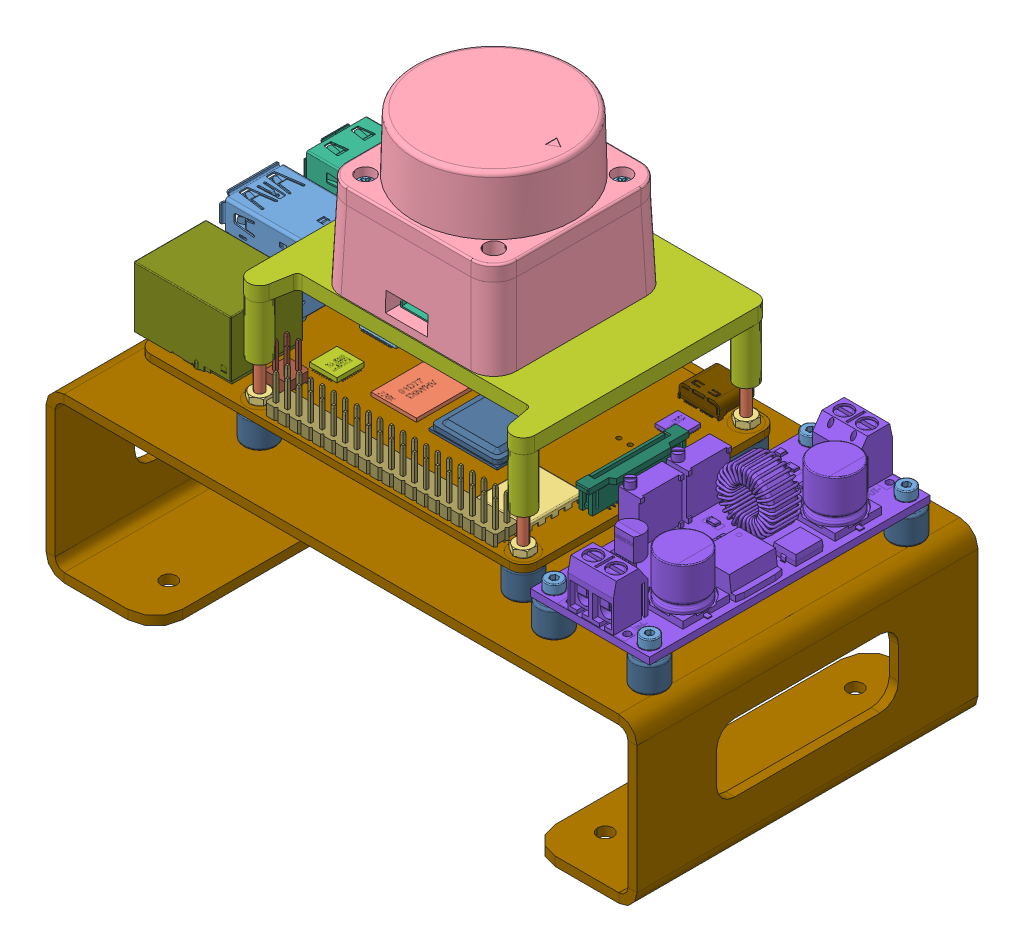
SolidWorks assembly 3rdFloorAssembly, configuration Default. Lengths in mm.
Overall size (130 100.19 75).
53 component instances, 28 part files, 56 mates.
Components (placement in the parent):
- socket head cap screw 4762_din-1: socket head cap screw 4762_din [EN ISO 4762 M2 x 12 - 12S] at (37.5 45.65 -28.25) x (0 -1 0) z (0 0 1) size (14 3.8 3.8)
- socket head cap screw 4762_din-2: socket head cap screw 4762_din [EN ISO 4762 M2 x 12 - 12S] at (58.5 45.65 -28.25) x (0 -1 0) z (0 0 1) size (14 3.8 3.8)
- socket head cap screw 4762_din-3: socket head cap screw 4762_din [EN ISO 4762 M2 x 12 - 12S] at (58.5 45.65 28.25) x (0 -1 0) z (0 0 1) size (14 3.8 3.8)
- socket head cap screw 4762_din-4: socket head cap screw 4762_din [EN ISO 4762 M2 x 12 - 12S] at (37.5 45.65 28.25) x (0 -1 0) z (0 0 1) size (14 3.8 3.8)
- socket head cap screw_iso-1: socket head cap screw_iso [ISO 4762 M2 x 20 - 20C] at (-31 32 -24.5) x (0 1 0) z (0 0 1) size (22 3.8 3.8)
- socket head cap screw_iso-2: socket head cap screw_iso [ISO 4762 M2 x 20 - 20C] at (-31 32 24.5) x (0 1 0) z (0 0 1) size (22 3.8 3.8)
- socket head cap screw_iso-3: socket head cap screw_iso [ISO 4762 M2 x 20 - 20C] at (27 32 -24.5) x (0 1 0) z (0 0 1) size (22 3.8 3.8)
- socket head cap screw_iso-4: socket head cap screw_iso [ISO 4762 M2 x 20 - 20C] at (27 32 24.5) x (0 1 0) z (0 0 1) size (22 3.8 3.8)
- hex nut style 1 gradeab_iso-1: hex nut style 1 gradeab_iso [ISO - 4032 - M2 - W - C] at (-31 45.19 -24.5) x (1 0 0) z (0 1 0) size (4 4.62 1.6)
- hex nut style 1 gradeab_iso-2: hex nut style 1 gradeab_iso [ISO - 4032 - M2 - W - C] at (27 45.19 -24.5) x (1 0 0) z (0 1 0) size (4 4.62 1.6)
- hex nut style 1 gradeab_iso-3: hex nut style 1 gradeab_iso [ISO - 4032 - M2 - W - C] at (-31 45.19 24.5) x (1 0 0) z (0 1 0) size (4 4.62 1.6)
- hex nut style 1 gradeab_iso-4: hex nut style 1 gradeab_iso [ISO - 4032 - M2 - W - C] at (27 45.19 24.5) x (1 0 0) z (0 1 0) size (4 4.62 1.6)
- hex nut style 1 gradeab_iso-5: hex nut style 1 gradeab_iso [ISO - 4032 - M2 - W - C] at (58.5 32.4 -28.25) x (1 0 0) z (0 -1 0) size (4 4.62 1.6)
- hex nut style 1 gradeab_iso-6: hex nut style 1 gradeab_iso [ISO - 4032 - M2 - W - C] at (37.5 32.4 -28.25) x (1 0 0) z (0 -1 0) size (4 4.62 1.6)
- hex nut style 1 gradeab_iso-7: hex nut style 1 gradeab_iso [ISO - 4032 - M2 - W - C] at (37.5 32.4 28.25) x (1 0 0) z (0 -1 0) size (4 4.62 1.6)
- hex nut style 1 gradeab_iso-8: hex nut style 1 gradeab_iso [ISO - 4032 - M2 - W - C] at (58.5 32.4 28.25) x (1 0 0) z (0 -1 0) size (4 4.62 1.6)
- LD06_Assembly-1: LD06_Assembly [Default] at (-60.828 42.1202 31.9351) x (0 0 -1) z (1 0 0) size (54 48.5 63)
  - LD06_LiDAR-1: LD06_LiDAR [Default] at (15.6414 21.3154 28.1688) size (38.59 33.3 38.59)
    - LD06_LiDAR-1: LD06_LiDAR [Default] at (16.3187 3.4544 28.6342) size (38.59 33.3 38.59)
    - JIS_B1111_M2x6.step-1: JIS_B1111_M2x6.step [Default] at (30.4187 21.1806 42.7342) x (1 0 0) z (0 1 0) size (3.5 3.5 7.3)
    - JIS_B1111_M2x6.step-2: JIS_B1111_M2x6.step [Default] at (2.2187 21.1806 14.5342) x (1 0 0) z (0 1 0) size (3.5 3.5 7.3)
    - jst-1.5mm-4P.step-1: jst-1.5mm-4P.step [Default] at (4.0237 7.1794 28.6342) x (0 0 -1) z (0 1 0) size (7.5 7.2 3.5)
  - LD06_PiBracket-1: LD06_PiBracket [Default] at (31.9351 21.5698 58.828) x (0 0 1) z (-1 0 0) size (63 27 54)
- dc-dc-5a-cc-merged-1: dc-dc-5a-cc-merged [Default] at (48 43.6 0) x (0 0 -1) z (1 0 0) size (61.7 17.87 26.2)
- Raspberry Pi 4 Model B-1: Raspberry Pi 4 Model B [Default] at (-12 42.8 0) x (-1 0 0) z (0 0 -1) size (88.99 19.9 58.4)
  - PCB, RPi4ModelB-1: PCB, RPi4ModelB [Default] at origin size (85 1.6 56)
  - Broadcom BCM2711B0 CPU, RPi4ModelB-1: Broadcom BCM2711B0 CPU, RPi4ModelB [Default] at (-13.25 0.8 -4.5) size (15 2.3 15)
  - 2.54 mm DUPONT MALE PIN HEADER, POE, 2X2, RPi4ModelB-1: 2.54 mm DUPONT MALE PIN HEADER, POE, 2X2, RPi4ModelB [Default] at (19 0.8 -18.5) size (5.08 11.3 5.08)
  - 2.54 mm DUPONT MALE PIN HEADER, IO, 2X20, RPi4ModelB-1: 2.54 mm DUPONT MALE PIN HEADER, IO, 2X20, RPi4ModelB [Default] at (-10 0.8 -24.5) size (50.8 11.3 5.08)
  - Camera Connector, RPi4ModelB-1: Camera Connector, RPi4ModelB [Default] at (4 0.8 16.5) x (0 0 -1) z (1 0 0) size (22.4 5.68 5.07)
  - Microphone Plug, RPi4ModelB-1: Microphone Plug, RPi4ModelB [Default] at (11.5 0.8 21.65) size (7.23 7.55 15)
  - Display Connector, RPi4ModelB-1: Display Connector, RPi4ModelB [Default] at (-38.5 0.8 0) x (0 0 1) z (-1 0 0) size (22.4 5.68 5.07)
  - Gigabit Ethernet Port, RPi4ModelB-1: Gigabit Ethernet Port, RPi4ModelB [Default] at (45.5 7.55 -17.75) x (0 0 -1) z (1 0 0) size (16.2 17.24 21.64)
  - Female Micro HDMI Connector, RPi4ModelB-2: Female Micro HDMI Connector, RPi4ModelB [Default] at (-3 0.8 27.3875) size (6.5 3.51 7.5)
  - Female Micro HDMI Connector, RPi4ModelB-3: Female Micro HDMI Connector, RPi4ModelB [Default] at (-16.5 0.8 27.3875) size (6.5 3.51 7.5)
  - Female USB Type C Connector, RPi4ModelB-1: Female USB Type C Connector, RPi4ModelB [Default] at (-31.3 0.8 26.5419) size (8.94 3.96 7.9)
  - 2X USB3.0 PORTS, RPi4ModelB-2: 2X USB3.0 PORTS, RPi4ModelB [Default] at (37.07 0.8 1) size (17.47 19.41 15.68)
  - 91D77 D9WHV 778K, 4 GB LPDDR4 SDRAM, RPi4ModelB-1: 91D77 D9WHV 778K, 4 GB LPDDR4 SDRAM, RPi4ModelB [Default] at (2.25 0.8 -4.5) size (10 0.8 14.5)
  - Cypress CYW43455 Wireless Module Cover, RPi4ModelB-1: Cypress CYW43455 Wireless Module Cover, RPi4ModelB [Default] at (-30.5 0.8 -14.5) size (11 1.6 13)
  - SD Card Slot, RPi4ModelB-1: SD Card Slot, RPi4ModelB [Default] at (-35.3 -0.8 0) x (0 0 -1) z (-1 0 0) size (11.95 1.45 11.4)
  - VIA VL805 PCIe USB 3.0 controller, RPi4ModelB-1: VIA VL805 PCIe USB 3.0 controller, RPi4ModelB [Default] at (17.5 0.8 4) size (8.8 0.8 8.8)
  - 2X USB2.0 PORTS, RPi4ModelB-1: 2X USB2.0 PORTS, RPi4ModelB [Default] at (37.065 0.65 19) size (17.87 19.16 15.33)
  - Broadcom BCM54213PE Gigabit Ethernet Transceiver, RPi4ModelB-1: Broadcom BCM54213PE Gigabit Ethernet Transceiver, RPi4ModelB [Default] at (16.5 0.8 -10) size (6.8 1 6.8)
  - MxL7704 Universal PMIC, RPi4ModelB-1: MxL7704 Universal PMIC, RPi4ModelB [Default] at (-32.5 0.8 16) size (5.4 0.8 5.4)
- 3rdFloor_Sheetmetal-1: 3rdFloor_Sheetmetal [Default] at (0 36 0) size (130 36 75)
- Spacer-1: Spacer [Default] at (37.5 36 -28.25) x (-0.470741 0 0.882271) z (-0.882271 0 -0.470741) size (7 6 7)
- Spacer-2: Spacer [Default] at (58.5 36 -28.25) x (0.784801 0 0.619748) z (-0.619748 0 0.784801) size (7 6 7)
- Spacer-3: Spacer [Default] at (-31 36 24.5) size (7 6 7)
- Spacer-4: Spacer [Default] at (37.5 36 28.25) x (0.517299 0 -0.855805) z (0.855805 0 0.517299) size (7 6 7)
- Spacer-5: Spacer [Default] at (58.5 36 28.25) size (7 6 7)
- Spacer-6: Spacer [Default] at (27 36.3 -24.5) x (-0.705828 0 0.708384) z (-0.708384 0 -0.705828) size (7 6 7)
- Spacer-7: Spacer [Default] at (27 36 24.5) x (0.999844 0 -0.017672) z (0.017672 0 0.999844) size (7 6 7)
- Spacer-8: Spacer [Default] at (-31 36 -24.5) x (-0.657111 0 -0.753794) z (0.753794 0 -0.657111) size (7 6 7)
Mates (geometry in assembly coordinates):
- Concentric98: concentric anti-aligned: cylinder of dc-dc-5a-cc-merged-1 through (37.5 43.65 -28.25) axis (0 -1 0) radius 2; cylinder of socket head cap screw 4762_din-1 through (37.5 77.4 -28.25) axis (0 1 0) radius 1.9
- Coincident95: coincident anti-aligned: plane of dc-dc-5a-cc-merged-1 through (37.5 43.65 -28.25) normal (0 1 0); plane of socket head cap screw 4762_din-1 through (39.4 43.65 -28.25) normal (0 -1 0)
- Concentric99: concentric aligned: cylinder of dc-dc-5a-cc-merged-1 through (58.5 43.65 -28.25) axis (0 1 0) radius 1.25; cylinder of socket head cap screw 4762_din-2 through (58.5 77.4 -28.25) axis (0 1 0) radius 1.9
- Coincident96: coincident anti-aligned: plane of dc-dc-5a-cc-merged-1 through (58.5 43.65 -28.25) normal (0 1 0); plane of socket head cap screw 4762_din-2 through (60.4 43.65 -28.25) normal (0 -1 0)
- Concentric100: concentric aligned: cylinder of dc-dc-5a-cc-merged-1 through (58.5 43.65 28.25) axis (0 1 0) radius 1.25; cylinder of socket head cap screw 4762_din-3 through (58.5 77.4 28.25) axis (0 1 0) radius 1.9
- Coincident97: coincident anti-aligned: plane of dc-dc-5a-cc-merged-1 through (58.5 43.65 28.25) normal (0 1 0); plane of socket head cap screw 4762_din-3 through (60.4 43.65 28.25) normal (0 -1 0)
- Concentric101: concentric aligned: cylinder of dc-dc-5a-cc-merged-1 through (37.5 43.65 28.25) axis (0 1 0) radius 1.25; cylinder of socket head cap screw 4762_din-4 through (37.5 77.4 28.25) axis (0 1 0) radius 1.9
- Coincident98: coincident anti-aligned: plane of dc-dc-5a-cc-merged-1 through (37.5 43.65 28.25) normal (0 1 0); plane of socket head cap screw 4762_din-4 through (39.4 43.65 28.25) normal (0 -1 0)
- Concentric1263: concentric anti-aligned: cylinder of 3rdFloor_Sheetmetal-1 through (-31 30.4645 -24.5) axis (0 1 0) radius 1.25; cylinder of socket head cap screw_iso-1 through (-31 0.25 -24.5) axis (0 -1 0) radius 1.9
- Coincident174: coincident anti-aligned: plane of 3rdFloor_Sheetmetal-1 through (0 34 0) normal (0 -1 0); plane of socket head cap screw_iso-1 through (-32.9 34 -24.5) normal (0 1 0)
- Concentric1264: concentric anti-aligned: cylinder of 3rdFloor_Sheetmetal-1 through (-31 30.4645 24.5) axis (0 1 0) radius 1.25; cylinder of socket head cap screw_iso-2 through (-31 0.25 24.5) axis (0 -1 0) radius 1.9
- Coincident175: coincident anti-aligned: plane of 3rdFloor_Sheetmetal-1 through (0 34 0) normal (0 -1 0); plane of socket head cap screw_iso-2 through (-32.9 34 24.5) normal (0 1 0)
- Concentric1265: concentric anti-aligned: cylinder of 3rdFloor_Sheetmetal-1 through (27 30.4645 -24.5) axis (0 1 0) radius 1.25; cylinder of socket head cap screw_iso-3 through (27 0.25 -24.5) axis (0 -1 0) radius 1.9
- Coincident176: coincident anti-aligned: plane of 3rdFloor_Sheetmetal-1 through (0 34 0) normal (0 -1 0); plane of socket head cap screw_iso-3 through (25.1 34 -24.5) normal (0 1 0)
- Concentric1266: concentric anti-aligned: cylinder of 3rdFloor_Sheetmetal-1 through (27 30.4645 24.5) axis (0 1 0) radius 1.25; cylinder of socket head cap screw_iso-4 through (27 0.25 24.5) axis (0 -1 0) radius 1.9
- Coincident177: coincident anti-aligned: plane of 3rdFloor_Sheetmetal-1 through (0 34 0) normal (0 -1 0); plane of socket head cap screw_iso-4 through (25.1 34 24.5) normal (0 1 0)
- Concentric1267: concentric aligned: cylinder of Raspberry Pi 4 Model B-1/PCB, RPi4ModelB-1 through (-31 43.6 -24.5) axis (0 1 0) radius 1.35; cylinder of hex nut style 1 gradeab_iso-1 through (-31 20.1525 -24.5) axis (0 1 0) radius 1
- Coincident178: coincident anti-aligned: plane of Raspberry Pi 4 Model B-1/PCB, RPi4ModelB-1 through (-31 43.59 -24.5) normal (0 1 0); plane of hex nut style 1 gradeab_iso-1 through (-35 43.59 -24.5) normal (0 -1 0)
- Distance5: distance = 6.5 mm anti-aligned: plane of LD06_Assembly-1/LD06_PiBracket-1 through (-31 51.69 -24.5) normal (0 -1 0); plane of hex nut style 1 gradeab_iso-1 through (-35 45.19 -24.5) normal (0 1 0)
- Concentric1268: concentric aligned: cylinder of Raspberry Pi 4 Model B-1/PCB, RPi4ModelB-1 through (27 43.6 -24.5) axis (0 1 0) radius 1.35; cylinder of hex nut style 1 gradeab_iso-2 through (27 20.1525 -24.5) axis (0 1 0) radius 1
- Coincident179: coincident anti-aligned: plane of Raspberry Pi 4 Model B-1/PCB, RPi4ModelB-1 through (27 43.59 -24.5) normal (0 1 0); plane of hex nut style 1 gradeab_iso-2 through (23 43.59 -24.5) normal (0 -1 0)
- Concentric1269: concentric aligned: cylinder of Raspberry Pi 4 Model B-1/PCB, RPi4ModelB-1 through (-31 43.6 24.5) axis (0 1 0) radius 1.35; cylinder of hex nut style 1 gradeab_iso-3 through (-31 20.1525 24.5) axis (0 1 0) radius 1
- Coincident180: coincident anti-aligned: plane of Raspberry Pi 4 Model B-1/PCB, RPi4ModelB-1 through (-31 43.59 24.5) normal (0 1 0); plane of hex nut style 1 gradeab_iso-3 through (-35 43.59 24.5) normal (0 -1 0)
- Concentric1270: concentric aligned: cylinder of Raspberry Pi 4 Model B-1/PCB, RPi4ModelB-1 through (27 43.6 24.5) axis (0 1 0) radius 1.35; cylinder of hex nut style 1 gradeab_iso-4 through (27 20.1525 24.5) axis (0 1 0) radius 1
- Coincident181: coincident anti-aligned: plane of Raspberry Pi 4 Model B-1/PCB, RPi4ModelB-1 through (27 43.59 24.5) normal (0 1 0); plane of hex nut style 1 gradeab_iso-4 through (23 43.59 24.5) normal (0 -1 0)
- Concentric1276: concentric anti-aligned: cylinder of 3rdFloor_Sheetmetal-1 through (58.5 30.4645 -28.25) axis (0 1 0) radius 1.25; cylinder of hex nut style 1 gradeab_iso-5 through (58.5 57.4375 -28.25) axis (0 -1 0) radius 1
- Coincident190: coincident anti-aligned: plane of 3rdFloor_Sheetmetal-1 through (0 34 0) normal (0 -1 0); plane of hex nut style 1 gradeab_iso-5 through (54.5 34 -28.25) normal (0 1 0)
- Concentric1277: concentric anti-aligned: cylinder of 3rdFloor_Sheetmetal-1 through (37.5 30.4645 -28.25) axis (0 1 0) radius 1.25; cylinder of hex nut style 1 gradeab_iso-6 through (37.5 57.4375 -28.25) axis (0 -1 0) radius 1
- Coincident191: coincident anti-aligned: plane of 3rdFloor_Sheetmetal-1 through (0 34 0) normal (0 -1 0); plane of hex nut style 1 gradeab_iso-6 through (33.5 34 -28.25) normal (0 1 0)
- Concentric1278: concentric anti-aligned: cylinder of 3rdFloor_Sheetmetal-1 through (37.5 30.4645 28.25) axis (0 1 0) radius 1.25; cylinder of hex nut style 1 gradeab_iso-7 through (37.5 57.4375 28.25) axis (0 -1 0) radius 1
- Coincident192: coincident anti-aligned: plane of 3rdFloor_Sheetmetal-1 through (0 34 0) normal (0 -1 0); plane of hex nut style 1 gradeab_iso-7 through (33.5 34 28.25) normal (0 1 0)
- Concentric1279: concentric anti-aligned: cylinder of 3rdFloor_Sheetmetal-1 through (58.5 30.4645 28.25) axis (0 1 0) radius 1.25; cylinder of hex nut style 1 gradeab_iso-8 through (58.5 57.4375 28.25) axis (0 -1 0) radius 1
- Coincident193: coincident anti-aligned: plane of 3rdFloor_Sheetmetal-1 through (0 34 0) normal (0 -1 0); plane of hex nut style 1 gradeab_iso-8 through (54.5 34 28.25) normal (0 1 0)
- Concentric1242: concentric aligned: cylinder of LD06_Assembly-1/LD06_PiBracket-1 through (-31 51.69 -24.5) axis (0 1 0) radius 0.75; circle of Raspberry Pi 4 Model B-1/PCB, RPi4ModelB-1
- Concentric1243: concentric aligned: cylinder of LD06_Assembly-1/LD06_PiBracket-1 through (27 51.69 24.5) axis (0 1 0) radius 0.75; circle of Raspberry Pi 4 Model B-1/PCB, RPi4ModelB-1
- Coincident86: coincident anti-aligned: plane of dc-dc-5a-cc-merged-1 through (58.5 42 -28.25) normal (0 -1 0); plane of Spacer-2 through (58.5 42 -28.25) normal (0 1 0)
- Concentric92: concentric anti-aligned: cylinder of dc-dc-5a-cc-merged-1 through (58.5 43.65 -28.25) axis (0 1 0) radius 1.25; cylinder of Spacer-2 through (58.5 42 -28.25) axis (0 -1 0) radius 1.5
- Concentric93: concentric anti-aligned: cylinder of dc-dc-5a-cc-merged-1 through (37.5 43.65 -28.25) axis (0 1 0) radius 1.25; cylinder of Spacer-1 through (37.5 42 -28.25) axis (0 -1 0) radius 1.5
- Concentric1240: concentric anti-aligned: cylinder of Spacer-8 through (-31 42 -24.5) axis (0 -1 0) radius 1.5; cylinder of Raspberry Pi 4 Model B-1/PCB, RPi4ModelB-1 through (-31 43.6 -24.5) axis (0 1 0) radius 1.35
- Concentric1241: concentric anti-aligned: cylinder of Spacer-7 through (27 42 24.5) axis (0 -1 0) radius 1.5; cylinder of Raspberry Pi 4 Model B-1/PCB, RPi4ModelB-1 through (27 43.6 24.5) axis (0 1 0) radius 1.35
- Coincident149: coincident anti-aligned: plane of Spacer-8 through (-31 42 -24.5) normal (0 1 0); plane of Raspberry Pi 4 Model B-1/PCB, RPi4ModelB-1 through (-12 42 0) normal (0 -1 0)
- Coincident78: coincident anti-aligned: plane of 3rdFloor_Sheetmetal-1 through (0 36 0) normal (0 1 0); plane of Spacer-1 through (37.5 36 -28.25) normal (0 -1 0)
- Concentric82: concentric anti-aligned: cylinder of 3rdFloor_Sheetmetal-1 through (37.5 30.4645 -28.25) axis (0 1 0) radius 1.25; cylinder of Spacer-1 through (37.5 42 -28.25) axis (0 -1 0) radius 1.5
- Concentric83: concentric anti-aligned: cylinder of 3rdFloor_Sheetmetal-1 through (58.5 30.4645 -28.25) axis (0 1 0) radius 1.25; cylinder of Spacer-2 through (58.5 42 -28.25) axis (0 -1 0) radius 1.5
- Coincident79: coincident anti-aligned: plane of 3rdFloor_Sheetmetal-1 through (0 36 0) normal (0 1 0); plane of Spacer-2 through (58.5 36 -28.25) normal (0 -1 0)
- Concentric84: concentric anti-aligned: cylinder of 3rdFloor_Sheetmetal-1 through (27 30.4645 -24.5) axis (0 1 0) radius 1.25; cylinder of Spacer-6 through (27 42.3 -24.5) axis (0 -1 0) radius 1.5
- Coincident81: coincident anti-aligned: plane of 3rdFloor_Sheetmetal-1 through (0 36 0) normal (0 1 0); plane of Spacer-8 through (-31 36 -24.5) normal (0 -1 0)
- Concentric85: concentric anti-aligned: cylinder of 3rdFloor_Sheetmetal-1 through (-31 30.4645 -24.5) axis (0 1 0) radius 1.25; cylinder of Spacer-8 through (-31 42 -24.5) axis (0 -1 0) radius 1.5
- Coincident82: coincident anti-aligned: plane of 3rdFloor_Sheetmetal-1 through (0 36 0) normal (0 1 0); plane of Spacer-5 through (58.5 36 28.25) normal (0 -1 0)
- Concentric86: concentric anti-aligned: cylinder of 3rdFloor_Sheetmetal-1 through (58.5 30.4645 28.25) axis (0 1 0) radius 1.25; cylinder of Spacer-5 through (58.5 42 28.25) axis (0 -1 0) radius 1.5
- Coincident83: coincident anti-aligned: plane of 3rdFloor_Sheetmetal-1 through (0 36 0) normal (0 1 0); plane of Spacer-4 through (37.5 36 28.25) normal (0 -1 0)
- Concentric87: concentric anti-aligned: cylinder of 3rdFloor_Sheetmetal-1 through (37.5 30.4645 28.25) axis (0 1 0) radius 1.25; cylinder of Spacer-4 through (37.5 42 28.25) axis (0 -1 0) radius 1.5
- Coincident84: coincident anti-aligned: plane of 3rdFloor_Sheetmetal-1 through (0 36 0) normal (0 1 0); plane of Spacer-7 through (27 36 24.5) normal (0 -1 0)
- Concentric88: concentric anti-aligned: cylinder of 3rdFloor_Sheetmetal-1 through (27 30.4645 24.5) axis (0 1 0) radius 1.25; cylinder of Spacer-7 through (27 42 24.5) axis (0 -1 0) radius 1.5
- Coincident85: coincident anti-aligned: plane of 3rdFloor_Sheetmetal-1 through (0 36 0) normal (0 1 0); plane of Spacer-3 through (-31 36 24.5) normal (0 -1 0)
- Concentric89: concentric anti-aligned: cylinder of 3rdFloor_Sheetmetal-1 through (-31 30.4645 24.5) axis (0 1 0) radius 1.25; cylinder of Spacer-3 through (-31 42 24.5) axis (0 -1 0) radius 1.5
